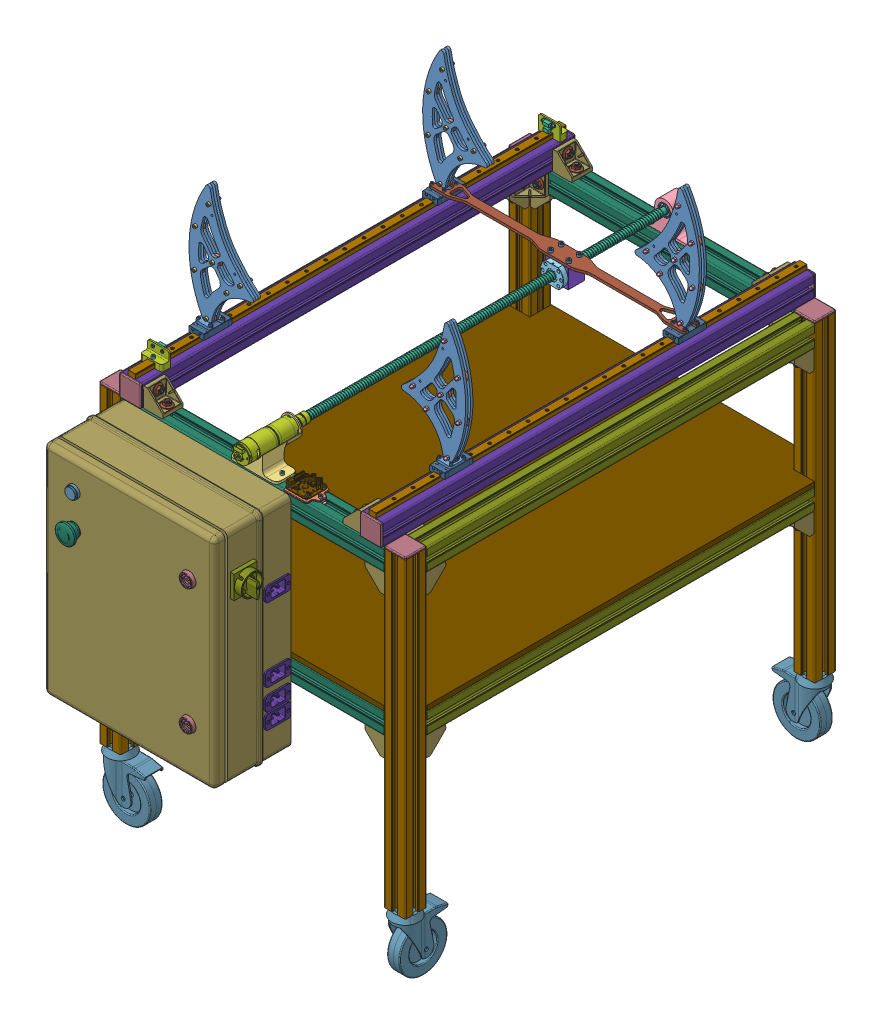
SolidWorks assembly Montaje_Eje_Z, configuration Predeterminado. Lengths in mm. (continued)
Mates (geometry in assembly coordinates): (continued)
- Coincidente66: coincident anti-aligned: plane of Viga_Union-1 through (23.5502 12.8322 -43.9995) normal (0 1 0); plane of socket head cap screw_iso2-9 through (265.2934 12.8322 -56.307) normal (0 -1 0)
- Coincidente67: coincident anti-aligned: plane of Viga_Union-1 through (23.5502 12.8322 -43.9995) normal (0 1 0); plane of socket head cap screw_iso2-6 through (290.2476 12.8322 -57.0348) normal (0 -1 0)
- Concéntrica25: concentric aligned: circle of Viga_Union-1; circle of socket head cap screw_iso-6
- Concéntrica27: concentric aligned: circle of HD16-1; circle of Viga_Union-1
- Concéntrica28: concentric aligned: cylinder of Viga_Union-1 through (43.5502 7.8322 -54.9995) axis (0 1 0) radius 2.55; cylinder of socket head cap screw_iso2-10 through (43.5502 49.5822 -54.9995) axis (0 1 0) radius 4.25
- Coincidente68: coincident anti-aligned: plane of Viga_Union-1 through (23.5502 12.8322 -43.9995) normal (0 1 0); plane of socket head cap screw_iso2-10 through (47.8002 12.8322 -54.9995) normal (0 -1 0)
- Concéntrica29: concentric aligned: cylinder of Viga_Union-1 through (43.5502 7.8322 -32.9995) axis (0 1 0) radius 2.55; cylinder of socket head cap screw_iso2-11 through (43.5502 49.5822 -32.9995) axis (0 1 0) radius 4.25
- Coincidente69: coincident anti-aligned: plane of Viga_Union-1 through (23.5502 12.8322 -43.9995) normal (0 1 0); plane of socket head cap screw_iso2-11 through (42.4407 12.8322 -37.1021) normal (0 -1 0)
- Concéntrica30: concentric aligned: cylinder of Viga_Union-1 through (5.5502 7.8322 -32.9995) axis (0 1 0) radius 2.55; cylinder of socket head cap screw_iso2-12 through (5.5502 49.5822 -32.9995) axis (0 1 0) radius 4.25
- Coincidente70: coincident anti-aligned: plane of Viga_Union-1 through (23.5502 12.8322 -43.9995) normal (0 1 0); plane of socket head cap screw_iso2-12 through (9.8002 12.8322 -32.9995) normal (0 -1 0)
- Concéntrica31: concentric aligned: cylinder of Viga_Union-1 through (5.5502 7.8322 -54.9995) axis (0 1 0) radius 2.55; cylinder of socket head cap screw_iso2-13 through (5.5502 49.5822 -54.9995) axis (0 1 0) radius 4.25
- Coincidente71: coincident anti-aligned: plane of Viga_Union-1 through (23.5502 12.8322 -43.9995) normal (0 1 0); plane of socket head cap screw_iso2-13 through (9.8002 12.8322 -54.9995) normal (0 -1 0)
- Coincidente78: coincident anti-aligned: line of Montaje_Mesa.CATProduct-1/P45L_N10_B_550.CATPart-1 through (-251.45 -58.9678 608.5586) axis (1 0 0); line of Armario-1/Caja-1 through (94.55 -58.9678 608.5586) axis (-1 0 0)
- Coincidente80: coincident aligned: line of Montaje_Mesa.CATProduct-1/P45L_N10_B_550.CATPart-1 through (-251.45 -58.9678 608.5586) axis (0 -1 0); line of Armario-1/Caja-1 through (-251.45 -68.9678 608.5586) axis (0 -1 0)
- Distancia14: distance = 22.5 mm: point of Montaje_Pata_Robot.CATProduct-3/Tuerca_Tornillo.CATProduct-4/1587_M4_Tuerca_Ciega.CATPart-1; plane of Montaje_Mesa.CATProduct-1/Montaje_Carril.CATProduct-2/P45L_N10_B_900.CATPart-1 through (-250.4501 -39.5678 608.4085) normal (-1 0 0)
- Distancia15: distance = 483.5249 mm: point of Montaje_Pata_Robot.CATProduct-1/Pata_Ext.CATPart-2; point of Montaje_Pata_Robot.CATProduct-3/Pata_Ext.CATPart-1
- Concéntrica32: concentric aligned: cylinder of MGN15C-1 through (287.5502 7.8322 456.5005) axis (0 1 0) radius 1.25; circle of Sujección-1
- Coincidente84: coincident anti-aligned: plane of MGN15C-1 through (275.0502 7.8322 465.7005) normal (0 1 0); plane of Sujección-1 through (275.0502 7.8322 444.0005) normal (0 -1 0)
- Concéntrica33: concentric anti-aligned: circle of MGN15C-1; circle of Sujección-1
- Concéntrica34: concentric aligned: circle of MGN15C-4; circle of Sujección-2
- Coincidente85: coincident anti-aligned: plane of MGN15C-4 through (-227.9501 7.8323 465.7005) normal (0 1 0); plane of Sujección-2 through (-227.9501 7.8323 444.0005) normal (0 -1 0)
- Concéntrica35: concentric aligned: circle of MGN15C-4; circle of Sujección-2
- Concéntrica44: concentric anti-aligned: cylinder of Sujección-1 through (287.5502 12.8322 456.5005) axis (0 -1 0) radius 1.55; cylinder of socket head cap screw_iso2-23 through (287.5502 47.5822 456.5005) axis (0 1 0) radius 2.75
- Coincidente94: coincident anti-aligned: plane of Sujección-1 through (275.0502 12.8322 444.0005) normal (0 1 0); plane of socket head cap screw_iso2-23 through (290.3002 12.8322 456.5005) normal (0 -1 0)
- Concéntrica45: concentric anti-aligned: cylinder of Sujección-1 through (287.5502 12.8322 431.5005) axis (0 -1 0) radius 1.55; cylinder of socket head cap screw_iso2-24 through (287.5502 47.5822 431.5005) axis (0 1 0) radius 2.75
- Coincidente95: coincident anti-aligned: plane of Sujección-1 through (275.0502 12.8322 444.0005) normal (0 1 0); plane of socket head cap screw_iso2-24 through (290.3002 12.8322 431.5005) normal (0 -1 0)
- Concéntrica46: concentric anti-aligned: cylinder of Sujección-1 through (262.5502 12.8322 456.5005) axis (0 -1 0) radius 1.55; cylinder of socket head cap screw_iso2-25 through (262.5502 47.5822 456.5005) axis (0 1 0) radius 2.75
- Coincidente96: coincident anti-aligned: plane of Sujección-1 through (275.0502 12.8322 444.0005) normal (0 1 0); plane of socket head cap screw_iso2-25 through (265.3002 12.8322 456.5005) normal (0 -1 0)
- Concéntrica47: concentric anti-aligned: cylinder of Sujección-1 through (262.5502 12.8322 431.5005) axis (0 -1 0) radius 1.55; cylinder of socket head cap screw_iso2-26 through (262.5502 47.5822 431.5005) axis (0 1 0) radius 2.75
- Coincidente97: coincident anti-aligned: plane of Sujección-1 through (275.0502 12.8322 444.0005) normal (0 1 0); plane of socket head cap screw_iso2-26 through (265.3002 12.8322 431.5005) normal (0 -1 0)
- Concéntrica48: concentric anti-aligned: cylinder of Sujección-2 through (-240.4501 12.8323 456.5005) axis (0 -1 0) radius 1.55; cylinder of socket head cap screw_iso2-27 through (-240.4501 47.5823 456.5005) axis (0 1 0) radius 2.75
- Coincidente98: coincident anti-aligned: plane of Sujección-2 through (-227.9501 12.8323 444.0005) normal (0 1 0); plane of socket head cap screw_iso2-27 through (-237.7001 12.8323 456.5005) normal (0 -1 0)
- Concéntrica49: concentric anti-aligned: cylinder of Sujección-2 through (-215.4501 12.8323 456.5005) axis (0 -1 0) radius 1.55; cylinder of socket head cap screw_iso2-28 through (-215.4501 47.5823 456.5005) axis (0 1 0) radius 2.75
- Coincidente99: coincident anti-aligned: plane of Sujección-2 through (-227.9501 12.8323 444.0005) normal (0 1 0); plane of socket head cap screw_iso2-28 through (-212.7001 12.8323 456.5005) normal (0 -1 0)
- Concéntrica50: concentric anti-aligned: cylinder of Sujección-2 through (-240.4501 12.8323 431.5005) axis (0 -1 0) radius 1.55; cylinder of socket head cap screw_iso2-29 through (-240.4501 47.5823 431.5005) axis (0 1 0) radius 2.75
- Coincidente100: coincident anti-aligned: plane of Sujección-2 through (-227.9501 12.8323 444.0005) normal (0 1 0); plane of socket head cap screw_iso2-29 through (-237.7001 12.8323 431.5005) normal (0 -1 0)
- Concéntrica51: concentric anti-aligned: cylinder of Sujección-2 through (-215.4501 12.8323 431.5005) axis (0 -1 0) radius 1.55; cylinder of socket head cap screw_iso2-30 through (-215.4501 47.5823 431.5005) axis (0 1 0) radius 2.75
- Coincidente101: coincident anti-aligned: plane of Sujección-2 through (-227.9501 12.8323 444.0005) normal (0 1 0); plane of socket head cap screw_iso2-30 through (-212.7001 12.8323 431.5005) normal (0 -1 0)
- Coincidente102: coincident anti-aligned: plane of Montaje_Mesa.CATProduct-1/P45L_N10_B_550.CATPart-1 through (-251.45 -55.9678 579.9585) normal (0 1 0); plane of Soporte_PCB_Motor_Z-1 through (114.6751 -55.9678 585.7153) normal (0 -1 0)
- Distancia18: distance = 1 mm aligned: plane of PCB_Control_Motores_V2.catpart-1 through (138.6751 -49.5208 568.0555) normal (1 0 0); plane of Soporte_PCB_Motor_Z-1 through (139.6751 -52.9678 611.0585) normal (1 0 0)
- Coincidente116: coincident anti-aligned: plane of Montaje_Mesa.CATProduct-1/P45L_N10_B_550.CATPart-1 through (-251.45 -57.7679 591.0585) normal (0 0 -1); plane of bosch_3842530281_56mh0c106byol9t07uu6uwj7k-1 through (84.6751 -61.9328 591.0585) normal (0 0 1)
- Coincidente117: coincident aligned: plane of Montaje_Mesa.CATProduct-1/P45L_N10_B_550.CATPart-1 through (-251.45 -55.9678 579.9585) normal (0 1 0); plane of bosch_3842530281_56mh0c106byol9t07uu6uwj7k-1 through (84.6751 -55.9678 586.0585) normal (0 1 0)
- Coincidente118: coincident aligned: plane of Montaje_Mesa.CATProduct-1/P45L_N10_B_550.CATPart-1 through (-251.45 -55.9678 579.9585) normal (0 1 0); plane of bosch_3842530281_56mh0c106byol9t07uu6uwj7k-2 through (144.6751 -55.9678 586.0585) normal (0 1 0)
- Coincidente119: coincident anti-aligned: plane of Montaje_Mesa.CATProduct-1/P45L_N10_B_550.CATPart-1 through (-251.45 -57.7679 591.0585) normal (0 0 -1); plane of bosch_3842530281_56mh0c106byol9t07uu6uwj7k-2 through (144.6751 -61.9328 591.0585) normal (0 0 1)
- Concéntrica63: concentric anti-aligned: circle of Soporte_PCB_Motor_Z-1; circle of bosch_3842530281_56mh0c106byol9t07uu6uwj7k-2
- Concéntrica64: concentric anti-aligned: circle of Soporte_PCB_Motor_Z-1; circle of bosch_3842530281_56mh0c106byol9t07uu6uwj7k-1
- Concéntrica65: concentric anti-aligned: cylinder of Soporte_PCB_Motor_Z-1 through (144.6751 -52.9678 586.0585) axis (0 -1 0) radius 2.05; cylinder of socket head cap screw_iso-31 through (144.6751 -17.2178 586.0585) axis (0 1 0) radius 3.5
- Coincidente121: coincident anti-aligned: plane of Soporte_PCB_Motor_Z-1 through (114.6751 -52.9678 585.7153) normal (0 1 0); plane of socket head cap screw_iso-31 through (148.1751 -52.9678 586.0585) normal (0 -1 0)
- Concéntrica66: concentric aligned: cylinder of bosch_3842530281_56mh0c106byol9t07uu6uwj7k-1 through (84.6751 -60.3178 586.0585) axis (0 1 0) radius 1.65; cylinder of socket head cap screw_iso-33 through (84.6751 -17.2178 586.0585) axis (0 1 0) radius 3.5
- Coincidente123: coincident anti-aligned: plane of Soporte_PCB_Motor_Z-1 through (114.6751 -52.9678 585.7153) normal (0 1 0); plane of socket head cap screw_iso-33 through (88.1751 -52.9678 586.0585) normal (0 -1 0)
- Concéntrica69: concentric aligned: circle of Soporte_PCB_Motor_Z-1; circle of hexa csunk flathd screw_iso-1
- Coincidente124: coincident anti-aligned: plane of Montaje_Mesa.CATProduct-1/P45L_N10_B_550.CATPart-1 through (-251.45 -55.9678 579.9585) normal (0 1 0); plane of hexa csunk flathd screw_iso-1 through (133.4451 -55.9678 604.7785) normal (0 -1 0)
- Coincidente125: coincident anti-aligned: plane of Montaje_Mesa.CATProduct-1/P45L_N10_B_550.CATPart-1 through (-251.45 -55.9678 579.9585) normal (0 1 0); plane of hexa csunk flathd screw_iso-4 through (133.4451 -55.9678 567.3685) normal (0 -1 0)
- Concéntrica73: concentric aligned: circle of Soporte_PCB_Motor_Z-1; circle of hexa csunk flathd screw_iso-4
- Coincidente126: coincident anti-aligned: plane of Montaje_Mesa.CATProduct-1/P45L_N10_B_550.CATPart-1 through (-251.45 -55.9678 579.9585) normal (0 1 0); plane of hexa csunk flathd screw_iso-2 through (96.0351 -55.9678 604.7785) normal (0 -1 0)
- Concéntrica74: concentric aligned: circle of Soporte_PCB_Motor_Z-1; circle of hexa csunk flathd screw_iso-2
- Coincidente127: coincident anti-aligned: plane of Montaje_Mesa.CATProduct-1/P45L_N10_B_550.CATPart-1 through (-251.45 -55.9678 579.9585) normal (0 1 0); plane of hexa csunk flathd screw_iso-5 through (96.0351 -55.9678 567.3685) normal (0 -1 0)
- Concéntrica75: concentric anti-aligned: cylinder of Soporte_PCB_Motor_Z-1 through (96.0351 -52.9678 567.3685) axis (0 -1 0) radius 1.55; circle of hexa csunk flathd screw_iso-5
- Concéntrica77: concentric aligned: cone of hexa csunk flathd screw_iso-2 through (96.0351 -44.1298 604.7785) axis (0 1 0); cylinder of hex thin nut chamfered gradeab_iso-1 through (96.0351 -71.1668 604.7785) axis (0 1 0) radius 1.5
- Coincidente129: coincident anti-aligned: plane of PCB_Control_Motores_V2.catpart-1 through (93.4611 -47.9293 564.8455) normal (0 1 0); plane of hex thin nut chamfered gradeab_iso-1 through (98.4859 -47.9293 602.7595) normal (0 -1 0)
- Concéntrica78: concentric aligned: cylinder of PCB_Control_Motores_V2.catpart-1 through (133.4739 -49.5208 604.6517) axis (0 1 0) radius 1.65; cylinder of hex thin nut chamfered gradeab_iso-2 through (133.4739 -71.1668 604.6517) axis (0 1 0) radius 1.5
- Coincidente130: coincident anti-aligned: plane of PCB_Control_Motores_V2.catpart-1 through (93.4611 -47.9293 564.8455) normal (0 1 0); plane of hex thin nut chamfered gradeab_iso-2 through (133.4739 -47.9293 601.4762) normal (0 -1 0)
- Concéntrica79: concentric aligned: cylinder of PCB_Control_Motores_V2.catpart-1 through (133.4739 -49.5208 567.2883) axis (0 1 0) radius 1.65; cylinder of hex thin nut chamfered gradeab_iso-3 through (133.4739 -71.1668 567.2883) axis (0 1 0) radius 1.5
- Coincidente131: coincident anti-aligned: plane of PCB_Control_Motores_V2.catpart-1 through (93.4611 -47.9293 564.8455) normal (0 1 0); plane of hex thin nut chamfered gradeab_iso-3 through (133.4739 -47.9293 564.1128) normal (0 -1 0)
- Concéntrica80: concentric aligned: cylinder of PCB_Control_Motores_V2.catpart-1 through (96.0597 -49.5208 567.2629) axis (0 1 0) radius 1.65; cylinder of hex thin nut chamfered gradeab_iso-4 through (96.0597 -71.1668 567.2629) axis (0 1 0) radius 1.5
- Coincidente132: coincident anti-aligned: plane of PCB_Control_Motores_V2.catpart-1 through (93.4611 -47.9293 564.8455) normal (0 1 0); plane of hex thin nut chamfered gradeab_iso-4 through (96.0597 -47.9293 564.0874) normal (0 -1 0)
- Coincidente134: coincident anti-aligned: plane of Montaje_Mesa.CATProduct-1/P45L_N10_B_550.CATPart-1 through (-251.45 -55.9678 579.9585) normal (0 1 0); plane of Soporte_Motor_Eje_Z-1 through (-25.4498 -55.9678 608.5585) normal (0 -1 0)
- Coincidente135: coincident aligned: plane of Montaje_Mesa.CATProduct-1/P45L_N10_B_550.CATPart-1 through (-251.45 -55.9678 579.9585) normal (0 1 0); plane of bosch_3842530281_56mh0c106byol9t07uu6uwj7k-4 through (-14.9498 -55.9678 586.0585) normal (0 1 0)
- Coincidente136: coincident anti-aligned: plane of Montaje_Mesa.CATProduct-1/P45L_N10_B_550.CATPart-1 through (-251.45 -57.7679 591.0585) normal (0 0 -1); plane of bosch_3842530281_56mh0c106byol9t07uu6uwj7k-4 through (-14.9498 -61.9328 591.0585) normal (0 0 1)
- Coincidente137: coincident anti-aligned: plane of Montaje_Mesa.CATProduct-1/P45L_N10_B_550.CATPart-1 through (-251.45 -57.7679 591.0585) normal (0 0 -1); plane of bosch_3842530281_56mh0c106byol9t07uu6uwj7k-3 through (64.0502 -61.9328 591.0585) normal (0 0 1)
- Coincidente138: coincident aligned: plane of Montaje_Mesa.CATProduct-1/P45L_N10_B_550.CATPart-1 through (-251.45 -55.9678 579.9585) normal (0 1 0); plane of bosch_3842530281_56mh0c106byol9t07uu6uwj7k-3 through (64.0502 -55.9678 586.0585) normal (0 1 0)
- Concéntrica81: concentric anti-aligned: circle of Soporte_Motor_Eje_Z-1; circle of bosch_3842530281_56mh0c106byol9t07uu6uwj7k-4
- Concéntrica82: concentric anti-aligned: circle of Soporte_Motor_Eje_Z-1; circle of bosch_3842530281_56mh0c106byol9t07uu6uwj7k-3
- Concéntrica85: concentric anti-aligned: circle of Motor_Tornillos-1/Motor_Tornillos.CATProduct-1/CHP-36GP-555.CATPart-1; circle of Soporte_Motor_Eje_Z-1
- Paralelo4: parallel: line of Motor_Tornillos-1/Motor_Tornillos.CATProduct-1/CHP-36GP-555.CATPart-1 through (15.7502 3.2472 639.5585) axis (0 -1 0); plane of Montaje_Mesa.CATProduct-1/Montaje_Carril.CATProduct-2/P45L_N10_B_900.CATPart-1 through (-205.45 -27.3677 608.4085) normal (1 0 0)
- Distancia19: distance = 25 mm aligned: plane of Motor_Tornillos-1/Motor_Tornillos.CATProduct-1/CHP-36GP-555.CATPart-1 through (24.5502 -12.1678 633.5585) normal (0 0 1); plane of Soporte_Motor_Eje_Z-1 through (24.5502 -12.1678 608.5585) normal (0 0 1)
- Concéntrica86: concentric aligned: cylinder of Soporte_Motor_Eje_Z-1 through (64.0502 -55.9678 586.0585) axis (0 1 0) radius 2.05; cylinder of socket head cap screw_iso-1 through (64.0502 -15.2178 586.0585) axis (0 1 0) radius 3.5
- Coincidente143: coincident anti-aligned: plane of Soporte_Motor_Eje_Z-1 through (45.5502 -50.9678 608.5585) normal (0 1 0); plane of socket head cap screw_iso-1 through (67.5502 -50.9678 586.0585) normal (0 -1 0)
- Concéntrica87: concentric aligned: cylinder of Soporte_Motor_Eje_Z-1 through (-14.9498 -55.9678 586.0585) axis (0 1 0) radius 2.05; cylinder of socket head cap screw_iso-2 through (-14.9498 -15.2178 586.0585) axis (0 1 0) radius 3.5
- Coincidente144: coincident anti-aligned: plane of Soporte_Motor_Eje_Z-1 through (-25.4498 -50.9678 608.5585) normal (0 1 0); plane of socket head cap screw_iso-2 through (-11.4498 -50.9678 586.0585) normal (0 -1 0)
- Concéntrica96: concentric anti-aligned: circle of Soporte_Motor_Eje_Z-1; circle of Soporte_Husillo_Eje_Z-1
- Coincidente148: coincident anti-aligned: plane of Montaje_Mesa.CATProduct-1/P45L_N10_B_550.CATPart-2 through (-251.45 -55.9678 -275.0416) normal (0 1 0); plane of Soporte_Husillo_Eje_Z-1 through (24.5502 -55.9678 -251.4416) normal (0 -1 0)
- Coincidente153: coincident anti-aligned: plane of Montaje_Mesa.CATProduct-1/P45L_N10_B_550.CATPart-2 through (-251.45 -61.6679 -273.9416) normal (0 0 1); plane of bosch_3842530281_56mh0c106byol9t07uu6uwj7k-6 through (-15.4498 -61.9328 -273.9416) normal (0 0 -1)
- Coincidente154: coincident anti-aligned: plane of Montaje_Mesa.CATProduct-1/P45L_N10_B_550.CATPart-2 through (-251.45 -61.6679 -273.9416) normal (0 0 1); plane of bosch_3842530281_56mh0c106byol9t07uu6uwj7k-5 through (64.5502 -61.9328 -273.9416) normal (0 0 -1)
- Coincidente155: coincident aligned: plane of Montaje_Mesa.CATProduct-1/P45L_N10_B_550.CATPart-2 through (-251.45 -55.9678 -275.0416) normal (0 1 0); plane of bosch_3842530281_56mh0c106byol9t07uu6uwj7k-5 through (64.5502 -55.9678 -268.9416) normal (0 1 0)
- Coincidente156: coincident aligned: plane of Montaje_Mesa.CATProduct-1/P45L_N10_B_550.CATPart-2 through (-251.45 -55.9678 -275.0416) normal (0 1 0); plane of bosch_3842530281_56mh0c106byol9t07uu6uwj7k-6 through (-15.4498 -55.9678 -268.9416) normal (0 1 0)
- Concéntrica97: concentric anti-aligned: circle of Soporte_Husillo_Eje_Z-1; circle of bosch_3842530281_56mh0c106byol9t07uu6uwj7k-5
- Concéntrica98: concentric anti-aligned: circle of Soporte_Husillo_Eje_Z-1; circle of bosch_3842530281_56mh0c106byol9t07uu6uwj7k-6
- Concéntrica99: concentric aligned: cylinder of Soporte_Husillo_Eje_Z-1 through (64.5502 -55.9678 -268.9416) axis (0 1 0) radius 2.05; cylinder of socket head cap screw_iso-3 through (64.5502 -15.2178 -268.9416) axis (0 1 0) radius 3.5
- Coincidente157: coincident anti-aligned: plane of Soporte_Husillo_Eje_Z-1 through (24.5502 -50.9678 -251.4416) normal (0 1 0); plane of socket head cap screw_iso-3 through (68.0502 -50.9678 -268.9416) normal (0 -1 0)
- Concéntrica100: concentric aligned: cylinder of Soporte_Husillo_Eje_Z-1 through (-15.4498 -55.9678 -268.9416) axis (0 1 0) radius 2.05; cylinder of socket head cap screw_iso-4 through (-15.4498 -15.2178 -268.9416) axis (0 1 0) radius 3.5
- Coincidente158: coincident anti-aligned: plane of Soporte_Husillo_Eje_Z-1 through (24.5502 -50.9678 -251.4416) normal (0 1 0); plane of socket head cap screw_iso-4 through (-11.9498 -50.9678 -268.9416) normal (0 -1 0)
- Concéntrica101: concentric anti-aligned: circle of Soporte_Husillo_Eje_Z-1; circle of 6000-Bearing-1
- Coincidente159: coincident aligned: plane of Soporte_Husillo_Eje_Z-1 through (24.5502 -53.4678 -251.4416) normal (0 0 1); plane of 6000-Bearing-1 through (24.5502 -12.1678 -251.4416) normal (0 0 1)
- Coincidente160: coincident aligned: plane of Soporte_Husillo_Eje_Z-1 through (24.5502 -53.4678 -286.4416) normal (0 0 -1); plane of 6000-Bearing-2 through (24.5502 -12.1678 -286.4416) normal (0 0 -1)
- Concéntrica102: concentric anti-aligned: circle of Soporte_Husillo_Eje_Z-1; circle of 6000-Bearing-2
- Coincidente164: coincident anti-aligned: plane of Montaje_Mesa.CATProduct-1/Montaje_Carril.CATProduct-2/P45L_N10_B_900.CATPart-1 through (-222.9501 -12.7678 608.4085) normal (-1 0 0); plane of bosch_3842530281_56mh0c106byol9t07uu6uwj7k-8 through (-222.9501 -16.9327 563.4085) normal (1 0 0)
- Coincidente165: coincident aligned: plane of Montaje_Mesa.CATProduct-1/Montaje_Carril.CATProduct-2/P45L_N10_B_900.CATPart-1 through (-234.0501 -10.9677 608.4085) normal (0 1 0); plane of bosch_3842530281_56mh0c106byol9t07uu6uwj7k-8 through (-227.9501 -10.9677 563.4085) normal (0 1 0)
- Coincidente166: coincident aligned: plane of Montaje_Mesa.CATProduct-1/Montaje_Carril.CATProduct-1/P45L_N10_B_900.CATPart-1 through (281.1501 -10.9677 -291.2916) normal (0 1 0); plane of bosch_3842530281_56mh0c106byol9t07uu6uwj7k-10 through (275.0502 -10.9677 -276.2916) normal (0 1 0)
- Coincidente168: coincident aligned: plane of Montaje_Mesa.CATProduct-1/Montaje_Carril.CATProduct-1/P45L_N10_B_900.CATPart-1 through (281.1501 -10.9677 -291.2916) normal (0 1 0); plane of bosch_3842530281_56mh0c106byol9t07uu6uwj7k-9 through (275.0502 -10.9677 563.7084) normal (0 1 0)
- Concéntrica110: concentric aligned: circle of MGN15 rail-3; circle of bosch_3842530281_56mh0c106byol9t07uu6uwj7k-7
- Concéntrica112: concentric anti-aligned: circle of MGN15 rail-2; circle of bosch_3842530281_56mh0c106byol9t07uu6uwj7k-9
- Concéntrica113: concentric anti-aligned: circle of MGN15 rail-2; circle of bosch_3842530281_56mh0c106byol9t07uu6uwj7k-10
- Coincidente169: coincident anti-aligned: plane of Montaje_Mesa.CATProduct-1/Montaje_Carril.CATProduct-2/P45L_N10_B_900.CATPart-1 through (-234.0501 -10.9677 608.4085) normal (0 1 0); plane of MGN15 rail-3 through (-235.2501 -10.9677 608.4085) normal (0 -1 0)
- Coincidente170: coincident: line of Montaje_Mesa.CATProduct-1/Montaje_Carril.CATProduct-2/P45L_N10_B_900.CATPart-1 through (-247.4501 -10.9677 -291.5915) axis (1 0 0); plane of MGN15 rail-3 through (-235.5501 -2.4677 -291.5915) normal (0 0 -1)
- Concéntrica114: concentric aligned: circle of HD16-1; circle of Soporte_Husillo_Eje_Z-1
- Concéntrica116: concentric anti-aligned: circle of MGN15 rail-3; circle of Soporte_FdC_Eje_Z-1
- Paralelo6: parallel aligned: plane of Montaje_Mesa.CATProduct-1/Montaje_Carril.CATProduct-2/P45L_N10_B_900.CATPart-1 through (-250.4501 -39.5678 608.4085) normal (-1 0 0); plane of Soporte_FdC_Eje_Z-1 through (-250.4501 0.5323 -272.5915) normal (-1 0 0)
- Coincidente178: coincident anti-aligned: plane of Montaje_Mesa.CATProduct-1/Montaje_Carril.CATProduct-2/P45L_N10_B_900.CATPart-1 through (-234.0501 -10.9677 608.4085) normal (0 1 0); plane of Soporte_FdC_Eje_Z-1 through (-205.4501 -10.9677 -272.5915) normal (0 -1 0)
- Coincidente179: coincident anti-aligned: plane of End_Stop-2 through (-227.9501 14.0323 -263.5915) normal (0 0 -1); plane of Soporte_FdC_Eje_Z-1 through (-250.4501 -0.9677 -263.5915) normal (0 0 1)
- Concéntrica122: concentric aligned: circle of End_Stop-2; circle of Soporte_FdC_Eje_Z-1
- Concéntrica123: concentric aligned: circle of End_Stop-2; circle of Soporte_FdC_Eje_Z-1
- Concéntrica124: concentric aligned: cylinder of Soporte_FdC_Eje_Z-1 through (-227.9501 -0.9677 -276.5915) axis (0 1 0) radius 2; cylinder of socket head cap screw_iso-5 through (-227.9501 37.7823 -276.5915) axis (0 1 0) radius 3.5
- Coincidente180: coincident anti-aligned: plane of Soporte_FdC_Eje_Z-1 through (-250.4501 2.0323 -281.5915) normal (0 1 0); plane of socket head cap screw_iso-5 through (-224.4501 2.0323 -276.5915) normal (0 -1 0)
- Concéntrica126: concentric anti-aligned: cylinder of End_Stop-2 through (-237.9501 14.0323 -262.7915) axis (0 0 -1) radius 1.5; cylinder of socket head cap screw_iso-8 through (-237.9501 14.0323 -227.2415) axis (0 0 1) radius 2.75
- Coincidente181: coincident anti-aligned: plane of End_Stop-2 through (-227.9501 14.0323 -261.9915) normal (0 0 1); plane of socket head cap screw_iso-8 through (-237.9501 16.7823 -261.9915) normal (0 0 -1)
- Concéntrica127: concentric anti-aligned: cylinder of End_Stop-2 through (-217.9501 14.0323 -262.7915) axis (0 0 -1) radius 1.5; cylinder of socket head cap screw_iso-9 through (-217.9501 14.0323 -227.2415) axis (0 0 1) radius 2.75
- Coincidente182: coincident anti-aligned: plane of End_Stop-2 through (-227.9501 14.0323 -261.9915) normal (0 0 1); plane of socket head cap screw_iso-9 through (-217.9501 16.7823 -261.9915) normal (0 0 -1)
- Concéntrica128: concentric anti-aligned: cylinder of End_Stop-1 through (-217.9501 14.0323 549.6085) axis (0 0 1) radius 1.5; cylinder of socket head cap screw_iso-10 through (-217.9501 14.0323 514.0585) axis (0 0 -1) radius 2.75
- Coincidente183: coincident anti-aligned: plane of End_Stop-1 through (-227.9501 14.0323 548.8085) normal (0 0 -1); plane of socket head cap screw_iso-10 through (-216.8967 11.4921 548.8085) normal (0 0 1)
- Concéntrica129: concentric anti-aligned: cylinder of End_Stop-1 through (-237.9501 14.0323 549.6085) axis (0 0 1) radius 1.5; cylinder of socket head cap screw_iso-11 through (-237.9501 14.0323 514.0585) axis (0 0 -1) radius 2.75
- Coincidente184: coincident anti-aligned: plane of End_Stop-1 through (-227.9501 14.0323 548.8085) normal (0 0 -1); plane of socket head cap screw_iso-11 through (-236.8967 11.4921 548.8085) normal (0 0 1)
- Concéntrica130: concentric anti-aligned: circle of MGN15 rail-3; circle of Soporte_FdC_Eje_Z-2
- Paralelo7: parallel aligned: plane of Montaje_Mesa.CATProduct-1/Montaje_Carril.CATProduct-2/P45L_N10_B_900.CATPart-1 through (-250.4501 -39.5678 608.4085) normal (-1 0 0); plane of Soporte_FdC_Eje_Z-2 through (-250.4501 0.5323 559.4085) normal (-1 0 0)
- Coincidente186: coincident anti-aligned: plane of Montaje_Mesa.CATProduct-1/Montaje_Carril.CATProduct-2/P45L_N10_B_900.CATPart-1 through (-234.0501 -10.9677 608.4085) normal (0 1 0); plane of Soporte_FdC_Eje_Z-2 through (-250.4501 -10.9677 559.4085) normal (0 -1 0)
- Coincidente187: coincident anti-aligned: plane of End_Stop-1 through (-227.9501 14.0323 550.4085) normal (0 0 1); plane of Soporte_FdC_Eje_Z-2 through (-205.4501 -0.9677 550.4085) normal (0 0 -1)
- Concéntrica131: concentric aligned: circle of socket head cap screw_iso-11; circle of Soporte_FdC_Eje_Z-2
- Concéntrica132: concentric aligned: circle of socket head cap screw_iso-10; circle of Soporte_FdC_Eje_Z-2
- Concéntrica133: concentric aligned: cylinder of Soporte_FdC_Eje_Z-2 through (-227.9501 -0.9677 563.4085) axis (0 1 0) radius 2; cylinder of socket head cap screw_iso-12 through (-227.9501 37.7823 563.4085) axis (0 1 0) radius 3.5
- Coincidente188: coincident anti-aligned: plane of Soporte_FdC_Eje_Z-2 through (-205.4501 2.0323 568.4085) normal (0 1 0); plane of socket head cap screw_iso-12 through (-224.4501 2.0323 563.4085) normal (0 -1 0)
- Concéntrica134: concentric anti-aligned: cylinder of Soporte_FdC_Eje_Z-2 through (-237.9501 14.0323 568.4085) axis (0 0 -1) radius 1.55; cylinder of hex thin nut gradeb_iso-1 through (-237.9501 14.0323 530.171) axis (0 0 1) radius 1.5
- Coincidente189: coincident anti-aligned: plane of Soporte_FdC_Eje_Z-2 through (-205.4501 2.0323 553.4085) normal (0 0 1); plane of hex thin nut gradeb_iso-1 through (-237.9501 17.2078 553.4085) normal (0 0 -1)
- Concéntrica135: concentric anti-aligned: cylinder of Soporte_FdC_Eje_Z-2 through (-217.9501 14.0323 568.4085) axis (0 0 -1) radius 1.55; cylinder of hex thin nut gradeb_iso-2 through (-217.9501 14.0323 530.171) axis (0 0 1) radius 1.5
- Coincidente190: coincident anti-aligned: plane of Soporte_FdC_Eje_Z-2 through (-205.4501 2.0323 553.4085) normal (0 0 1); plane of hex thin nut gradeb_iso-2 through (-217.9501 17.2078 553.4085) normal (0 0 -1)
- Concéntrica136: concentric aligned: cone of socket head cap screw_iso-8 through (-237.9501 14.0323 -269.9915) axis (0 0 -1); cylinder of hex thin nut gradeb_iso-3 through (-237.9501 14.0323 -243.354) axis (0 0 -1) radius 1.5
- Coincidente191: coincident anti-aligned: plane of Soporte_FdC_Eje_Z-1 through (-250.4501 2.0323 -266.5915) normal (0 0 -1); plane of hex thin nut gradeb_iso-3 through (-237.9502 17.2078 -266.5915) normal (0 0 1)
- Concéntrica137: concentric anti-aligned: cylinder of Soporte_FdC_Eje_Z-1 through (-217.9501 14.0323 -281.5915) axis (0 0 1) radius 1.55; cylinder of hex thin nut gradeb_iso-4 through (-217.9501 14.0323 -243.354) axis (0 0 -1) radius 1.5
- Coincidente192: coincident anti-aligned: plane of Soporte_FdC_Eje_Z-1 through (-250.4501 2.0323 -266.5915) normal (0 0 -1); plane of hex thin nut gradeb_iso-4 through (-217.9502 17.2078 -266.5915) normal (0 0 1)
